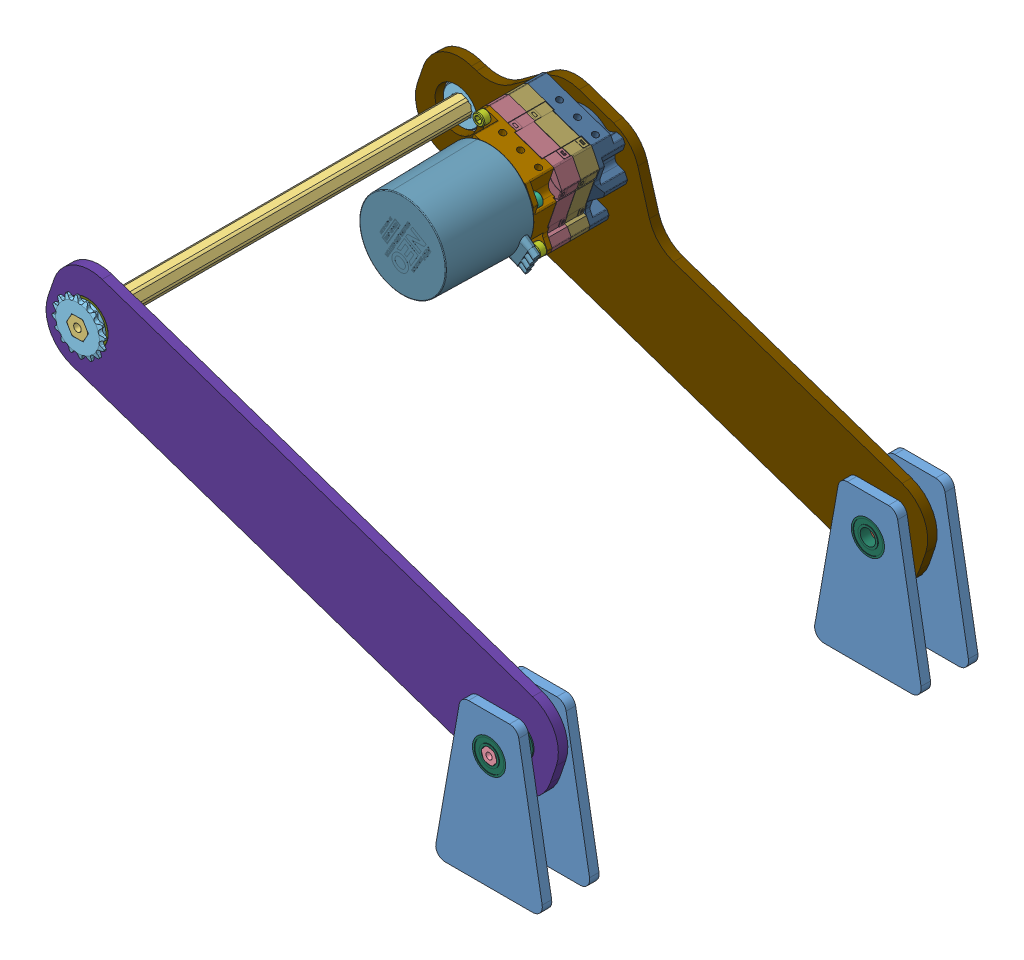
SolidWorks assembly intakeassembly, configuration Default. Lengths in mm.
Overall size (371.43 254.48 292.1).
35 component instances, 18 part files, 50 mates.
Components (placement in the parent):
- layout_sketch (2)-2: layout_sketch (2) [Default] at (16.0396 36.7133 123.2199) size (71.49 101.6 6.35)
- layout_sketch (2)-3: layout_sketch (2) [Default] at (16.0396 36.7133 -99.0301) size (71.49 101.6 6.35)
- 1_2thunderhex_1.5in-1: 1_2thunderhex_1.5in [Default] at (53.0044 112.9133 -556.2301) x (-0.618535 -0.785757 0) z (0 0 1) size (13.74 12.75 31.75)
- 1_2thunderhex_10.5in-1: 1_2thunderhex_10.5in [Default] at (-235.6241 210.8757 -308.5801) x (-0.456167 0.889894 0) z (0 0 1) size (13.74 12.75 266.7)
- 3_8thunderhex_1.5in-1: 3_8thunderhex_1.5in [Default] at (53.0044 112.9133 -295.8801) x (0.332678 -0.943041 0) z (0 0 1) size (10.24 9.53 38.1)
- 16T_#25_500_hex_hubbed_sprocket_217-2642-1: 16T_#25_500_hex_hubbed_sprocket_217-2642 [Default] at (-235.6241 210.8757 145.8259) x (-0.877701 0.479208 0) z (0 0 1) size (35.21 35.21 9.18)
- MAXPlanetary 2-Stage-1: MAXPlanetary 2-Stage [Default] at (-149.8677 235.4157 -51.4051) x (-0.946944 0.321399 0) z (0 0 -1) size (89.61 89.51 122.08)
  - MAXPlanetary 2-Stage.STEP-1: MAXPlanetary 2-Stage.STEP [Default] at origin size (89.61 89.51 122.08)
    - REV-25-2109_2-Stage (No Shaft, For NEO).STEP-1: REV-25-2109_2-Stage (No Shaft, For NEO).STEP [Default] at origin size (65.15 54.03 73.34)
      - REV-25-2107_2-Stage.STEP-1: REV-25-2107_2-Stage.STEP [Default] at (0 0 6.35) x (-1 0 0) z (0 0 -1) size (65.15 54.03 73.34)
        - #10 Socket Head Cap Screws_0.500in Long.STEP-1: #10 Socket Head Cap Screws_0.500in Long.STEP [Default] at (21.1355 14.0872 12.7) x (0.923728 0.383049 0) z (0.383049 -0.923728 0) size (7.94 17.53 7.94)
        - #10 Socket Head Cap Screws_0.500in Long.STEP-2: #10 Socket Head Cap Screws_0.500in Long.STEP [Default] at (-21.1355 -14.0872 12.7) x (0.923728 0.383049 0) z (0.383049 -0.923728 0) size (7.94 17.53 7.94)
        - #10 Socket Head Cap Screws_1.500in Long.STEP-1: #10 Socket Head Cap Screws_1.500in Long.STEP [Default] at (-26.9919 21.4312 0) x (0.777574 0.628792 0) z (-0.628792 0.777574 0) size (7.94 42.93 7.94)
        - #10 Socket Head Cap Screws_1.500in Long.STEP-2: #10 Socket Head Cap Screws_1.500in Long.STEP [Default] at (26.9919 -21.4312 0) x (0.777574 0.628792 0) z (-0.628792 0.777574 0) size (7.94 42.93 7.94)
        - #10-32 Button Head Cap Screws_0.500in Long.STEP-1: #10-32 Button Head Cap Screws_0.500in Long.STEP [Default] at (0 0 -35.2425) x (0.655967 -0.754789 0) z (-0.754789 -0.655967 0) size (9.17 15.27 9.17)
      - REV-21-2106.STEP-1: REV-21-2106.STEP [Default] at origin size (61.91 50.8 19.05)
      - REV-21-2104.STEP-1: REV-21-2104.STEP [Default] at (0 0 44.45) x (0 0 1) z (-1 0 0) size (23.2 50.8 61.92)
      - REV-21-2108.STEP-1: REV-21-2108.STEP [Default] at (0 0 7.0985) x (-0.554615 -0.832107 0) z (0 0 -1) size (25.4 25.4 14.94)
    - REV-21-2101.STEP-1: REV-21-2101.STEP [Default] at (0 0 28.575) size (61.91 50.8 16.85)
    - REV-21-2102.STEP-1: REV-21-2102.STEP [Default] at (0 0 15.875) size (61.91 50.8 16.85)
    - REV-21-1650.STEP-1: REV-21-1650.STEP [Default] at (0 0 -9.525) x (0.554615 0.832107 0) z (0 0 1) size (64.41 64.76 93.26)
- thunderhex_375_flanged_217-5829-1: thunderhex_375_flanged_217-5829 [Default] at (53.0044 112.9133 154.2079) x (0 0 1) z (-0.756545 -0.653942 0) size (7.11 24.61 24.61)
- thunderhex_375_flanged_217-5829-2: thunderhex_375_flanged_217-5829 [Default] at (53.0044 112.9133 -123.6681) x (0 0 -1) z (-0.718679 0.695342 0) size (7.11 24.61 24.61)
- thunderhex_flanged_217-4006-2: thunderhex_flanged_217-4006 [Default] at (-235.6241 210.8757 138.3012) x (-1 0 0) z (0 0 -1) size (31.12 31.12 7.94)
- layout_sketch (2)-4: layout_sketch (2) [Default] at (16.0396 36.7133 154.9699) size (71.49 101.6 6.35)
- layout_sketch (2)-5: layout_sketch (2) [Default] at (16.0396 36.7133 -130.7801) size (71.49 101.6 6.35)
- thunderhex_375_flanged_217-5829-3: thunderhex_375_flanged_217-5829 [Default] at (53.0044 112.9133 130.3319) x (0 0 -1) z (-0.959715 -0.280976 0) size (7.11 24.61 24.61)
- thunderhex_375_flanged_217-5829-5: thunderhex_375_flanged_217-5829 [Default] at (53.0044 112.9133 -99.7921) x (0 0 1) z (-0.999866 -0.016349 0) size (7.11 24.61 24.61)
- thunderhex_375_flanged_217-5829-6: thunderhex_375_flanged_217-5829 [Default] at (53.0044 112.9133 135.9199) x (0 0 1) z (-0.999379 0.03525 0) size (7.11 24.61 24.61)
- thunderhex_375_flanged_217-5829-7: thunderhex_375_flanged_217-5829 [Default] at (53.0044 112.9133 -105.3801) x (0 0 -1) z (-0.879404 0.476076 0) size (7.11 24.61 24.61)
- layout_sketch (1)-1: layout_sketch (1) [Default] at (63.5174 28.8757 142.2699) x (-0.946944 0.321399 0) z (0 0 -1) size (355.6 63.5 6.35)
- layout_sketch-1: layout_sketch [Default] at (63.5174 28.8757 -105.3801) x (-0.946944 0.321399 0) z (0 0 -1) size (355.6 107.95 6.35)
- 16T_#25_500_hex_hubbed_sprocket_217-2642-2: 16T_#25_500_hex_hubbed_sprocket_217-2642 [Default] at (-235.6241 210.8757 -115.2861) x (-1 0 0) z (0 0 -1) size (35.21 35.21 9.18)
- 16T_#25_500_hex_hubbed_sprocket_217-2642-3: 16T_#25_500_hex_hubbed_sprocket_217-2642 [Default] at (-149.8677 235.4157 -115.2861) x (-0.723016 -0.690831 0) z (0 0 -1) size (35.21 35.21 9.18)
- 1_2thunderhex_1.5in-2: 1_2thunderhex_1.5in [Default] at (-149.8677 235.4157 -543.5301) x (0.99729 -0.073573 0) z (0 0 1) size (13.74 12.75 31.75)
Mates (geometry in assembly coordinates):
- Parallel1: parallel aligned: line of layout_sketch (2)-2 through (23.6073 36.7133 129.5699) axis (1 0 0); line of layout_sketch (2)-3 through (23.6073 36.7133 -92.6801) axis (1 0 0)
- Parallel3: parallel aligned: plane of layout_sketch (2)-2 through (39.2827 138.3133 129.5699) normal (0 1 0); plane of layout_sketch (2)-3 through (39.2827 138.3133 -92.6801) normal (0 1 0)
- Distance1: distance = 222.25 mm aligned: plane of layout_sketch (2)-3 through (82.4016 43.0633 -92.6801) normal (0 0 1); plane of layout_sketch (2)-2 through (82.4016 43.0633 129.5699) normal (0 0 1)
- Coincident3: coincident aligned: plane of layout_sketch (2)-2 through (39.2827 138.3133 129.5699) normal (0 1 0); plane of layout_sketch (2)-3 through (39.2827 138.3133 -92.6801) normal (0 1 0)
- Coincident4: coincident aligned: plane of layout_sketch (2)-2 through (72.9797 133.0659 129.5699) normal (0.984808 0.173648 0); plane of layout_sketch (2)-3 through (72.9797 133.0659 -92.6801) normal (0.984808 0.173648 0)
- Parallel6: parallel aligned: plane of layout_sketch (2)-2 through (39.2827 138.3133 129.5699) normal (0 1 0); plane of layout_sketch (2)-4 through (39.2827 138.3133 161.3199) normal (0 1 0)
- Parallel7: parallel aligned: plane of layout_sketch (2)-2 through (72.9797 133.0659 129.5699) normal (0.984808 0.173648 0); plane of layout_sketch (2)-4 through (72.9797 133.0659 161.3199) normal (0.984808 0.173648 0)
- Coincident14: coincident aligned: plane of layout_sketch (2)-2 through (72.9797 133.0659 129.5699) normal (0.984808 0.173648 0); plane of layout_sketch (2)-4 through (72.9797 133.0659 161.3199) normal (0.984808 0.173648 0)
- Coincident15: coincident aligned: plane of layout_sketch (2)-2 through (39.2827 138.3133 129.5699) normal (0 1 0); plane of layout_sketch (2)-4 through (39.2827 138.3133 161.3199) normal (0 1 0)
- Coincident16: coincident aligned: plane of layout_sketch (2)-3 through (39.2827 138.3133 -92.6801) normal (0 1 0); plane of layout_sketch (2)-5 through (39.2827 138.3133 -124.4301) normal (0 1 0)
- Coincident17: coincident aligned: plane of layout_sketch (2)-3 through (72.9797 133.0659 -92.6801) normal (0.984808 0.173648 0); plane of layout_sketch (2)-5 through (72.9797 133.0659 -124.4301) normal (0.984808 0.173648 0)
- Coincident20: coincident aligned: plane of layout_sketch (2)-3 through (82.4016 43.0633 -92.6801) normal (0 0 1); plane of thunderhex_375_flanged_217-5829-5 through (52.8425 122.8179 -92.6801) normal (0 0 1)
- Concentric9: concentric aligned: cylinder of layout_sketch (2)-3 through (53.0044 112.9133 -92.6801) axis (0 0 -1) radius 11.1125; cylinder of thunderhex_375_flanged_217-5829-5 through (53.0044 112.9133 -99.7921) axis (0 0 -1) radius 5.125
- Coincident23: coincident aligned: plane of thunderhex_375_flanged_217-5829-2 through (46.1164 105.794 -130.7801) normal (0 0 -1); plane of layout_sketch (2)-5 through (82.4016 43.0633 -130.7801) normal (0 0 -1)
- Concentric10: concentric anti-aligned: cylinder of thunderhex_375_flanged_217-5829-2 through (53.0044 112.9133 -123.6681) axis (0 0 1) radius 5.125; cylinder of layout_sketch (2)-5 through (53.0044 112.9133 -124.4301) axis (0 0 -1) radius 11.1125
- Coincident27: coincident aligned: plane of layout_sketch (2)-2 through (82.4016 43.0633 123.2199) normal (0 0 -1); plane of thunderhex_375_flanged_217-5829-3 through (55.7878 103.4063 123.2199) normal (0 0 -1)
- Concentric13: concentric anti-aligned: cylinder of layout_sketch (2)-2 through (53.0044 112.9133 129.5699) axis (0 0 -1) radius 11.1125; cylinder of thunderhex_375_flanged_217-5829-3 through (53.0044 112.9133 130.3319) axis (0 0 1) radius 5.125
- Coincident31: coincident aligned: plane of thunderhex_375_flanged_217-5829-1 through (46.5265 120.4076 161.3199) normal (0 0 1); plane of layout_sketch (2)-4 through (82.4016 43.0633 161.3199) normal (0 0 1)
- Concentric15: concentric anti-aligned: cylinder of thunderhex_375_flanged_217-5829-1 through (53.0044 112.9133 154.2079) axis (0 0 -1) radius 5.125; circle of layout_sketch (2)-4
- Distance2: distance = 31.75 mm aligned: plane of layout_sketch (2)-2 through (82.4016 43.0633 129.5699) normal (0 0 1); plane of layout_sketch (2)-4 through (82.4016 43.0633 161.3199) normal (0 0 1)
- Distance3: distance = 31.75 mm aligned: plane of layout_sketch (2)-5 through (82.4016 43.0633 -124.4301) normal (0 0 1); plane of layout_sketch (2)-3 through (82.4016 43.0633 -92.6801) normal (0 0 1)
- Coincident34: coincident aligned: plane of 3_8thunderhex_1.5in-1 through (53.0044 112.9133 161.3199) normal (0 0 1); plane of layout_sketch (2)-4 through (82.4016 43.0633 161.3199) normal (0 0 1)
- Concentric16: concentric anti-aligned: cylinder of 3_8thunderhex_1.5in-1 through (53.0044 112.9133 -753.0801) axis (0 0 1) radius 2.1; cylinder of thunderhex_375_flanged_217-5829-1 through (53.0044 112.9133 154.2079) axis (0 0 -1) radius 5.125
- Coincident36: coincident aligned: plane of 1_2thunderhex_1.5in-1 through (88.5441 168.3684 -130.7801) normal (0 0 -1); plane of layout_sketch (2)-5 through (82.4016 43.0633 -130.7801) normal (0 0 -1)
- Concentric17: concentric aligned: cylinder of 1_2thunderhex_1.5in-1 through (53.0044 112.9133 -1013.4301) axis (0 0 1) radius 2.55; cylinder of thunderhex_375_flanged_217-5829-2 through (53.0044 112.9133 -123.6681) axis (0 0 1) radius 5.125
- Concentric18: concentric aligned: cylinder of 1_2thunderhex_1.5in-1 through (53.0044 112.9133 -1013.4301) axis (0 0 1) radius 2.55; cylinder of thunderhex_375_flanged_217-5829-7 through (53.0044 112.9133 -105.3801) axis (0 0 1) radius 5.125
- Concentric19: concentric anti-aligned: cylinder of 3_8thunderhex_1.5in-1 through (53.0044 112.9133 -753.0801) axis (0 0 1) radius 2.1; cylinder of thunderhex_375_flanged_217-5829-6 through (53.0044 112.9133 135.9199) axis (0 0 -1) radius 5.125
- Distance6: distance = 12.7 mm aligned: plane of thunderhex_375_flanged_217-5829-7 through (47.1457 102.0911 -105.3801) normal (0 0 1); plane of layout_sketch (2)-3 through (82.4016 43.0633 -92.6801) normal (0 0 1)
- Distance7: distance = 12.7 mm aligned: plane of layout_sketch (2)-2 through (82.4016 43.0633 123.2199) normal (0 0 -1); plane of thunderhex_375_flanged_217-5829-6 through (53.4382 125.2119 135.9199) normal (0 0 -1)
- Concentric20: concentric aligned: cylinder of thunderhex_375_flanged_217-5829-7 through (53.0044 112.9133 -105.3801) axis (0 0 1) radius 11.1125; cylinder of layout_sketch-1 through (53.0044 112.9133 -111.7301) axis (0 0 1) radius 11.1125
- Concentric21: concentric aligned: cylinder of 3_8thunderhex_1.5in-1 through (53.0044 112.9133 -753.0801) axis (0 0 1) radius 2.1; cylinder of layout_sketch (1)-1 through (53.0044 112.9133 135.9199) axis (0 0 1) radius 11.1125
- Parallel9: parallel aligned: plane of layout_sketch (1)-1 through (63.2089 142.9787 135.9199) normal (0.321399 0.946944 0); plane of layout_sketch-1 through (63.2089 142.9787 -111.7301) normal (0.321399 0.946944 0)
- Coincident47: coincident aligned: plane of thunderhex_375_flanged_217-5829-6 through (53.4382 125.2119 135.9199) normal (0 0 -1); plane of layout_sketch (1)-1 through (-237.6649 204.8626 135.9199) normal (0 0 -1)
- Coincident48: coincident aligned: plane of thunderhex_375_flanged_217-5829-7 through (47.1457 102.0911 -105.3801) normal (0 0 1); plane of layout_sketch-1 through (-237.6649 204.8626 -105.3801) normal (0 0 1)
- Concentric23: concentric aligned: cylinder of 1_2thunderhex_10.5in-1 through (-235.6241 210.8757 -765.7801) axis (0 0 1) radius 2.55; cylinder of layout_sketch (1)-1 through (-235.6241 210.8757 135.9199) axis (0 0 1) radius 14.2875
- Distance8: distance = 6.35 mm aligned: plane of 1_2thunderhex_10.5in-1 through (-235.6241 210.8757 148.6199) normal (0 0 1); plane of layout_sketch (1)-1 through (-237.6649 204.8626 142.2699) normal (0 0 1)
- Coincident51: coincident aligned: plane of thunderhex_flanged_217-4006-2 through (-235.6241 223.1632 142.2699) normal (0 0 1); plane of layout_sketch (1)-1 through (-237.6649 204.8626 142.2699) normal (0 0 1)
- Concentric24: concentric anti-aligned: cylinder of thunderhex_flanged_217-4006-2 through (-235.6241 210.8757 85.0522) axis (0 0 -1) radius 6.875; cylinder of layout_sketch (1)-1 through (-235.6241 210.8757 135.9199) axis (0 0 1) radius 14.2875
- Concentric26: concentric anti-aligned: cylinder of 16T_#25_500_hex_hubbed_sprocket_217-2642-1 through (-235.6241 210.8757 139.4442) axis (0 0 1) radius 12.7; cylinder of thunderhex_flanged_217-4006-2 through (-235.6241 210.8757 85.0522) axis (0 0 -1) radius 14.2875
- Concentric27: concentric aligned: circle of 16T_#25_500_hex_hubbed_sprocket_217-2642-1; circle of thunderhex_flanged_217-4006-2
- Coincident53: coincident aligned: plane of 1_2thunderhex_10.5in-1 through (-235.6241 210.8757 148.6199) normal (0 0 1); plane of 16T_#25_500_hex_hubbed_sprocket_217-2642-1 through (-235.6241 210.8757 148.6199) normal (0 0 1)
- Concentric28: concentric anti-aligned: cylinder of 1_2thunderhex_10.5in-1 through (-235.6241 210.8757 -765.7801) axis (0 0 1) radius 2.55; cylinder of 16T_#25_500_hex_hubbed_sprocket_217-2642-2 through (-235.6241 210.8757 -108.9043) axis (0 0 -1) radius 12.7
- Coincident55: coincident aligned: plane of 1_2thunderhex_10.5in-1 through (-200.0458 155.4454 -118.0801) normal (0 0 -1); plane of 16T_#25_500_hex_hubbed_sprocket_217-2642-2 through (-235.6241 210.8757 -118.0801) normal (0 0 -1)
- Coincident56: coincident anti-aligned: plane of MAXPlanetary 2-Stage-1/MAXPlanetary 2-Stage.STEP-1/REV-25-2109_2-Stage (No Shaft, For NEO).STEP-1/REV-21-2104.STEP-1 through (-149.8677 235.4157 -105.3801) normal (0 0 -1); plane of layout_sketch-1 through (-237.6649 204.8626 -105.3801) normal (0 0 1)
- Parallel10: parallel aligned: plane of MAXPlanetary 2-Stage-1/MAXPlanetary 2-Stage.STEP-1/REV-25-2109_2-Stage (No Shaft, For NEO).STEP-1/REV-21-2104.STEP-1 through (-165.7565 267.6316 -86.3301) normal (0.321399 0.946944 0); plane of layout_sketch-1 through (63.2089 142.9787 -111.7301) normal (0.321399 0.946944 0)
- Concentric29: concentric aligned: cylinder of MAXPlanetary 2-Stage-1/MAXPlanetary 2-Stage.STEP-1/REV-25-2109_2-Stage (No Shaft, For NEO).STEP-1/REV-25-2107_2-Stage.STEP-1/#10-32 Button Head Cap Screws_0.500in Long.STEP-1 through (-149.8677 235.4157 -92.3753) axis (0 0 1) radius 2.413; cylinder of layout_sketch-1 through (-149.8677 235.4157 -111.7301) axis (0 0 1) radius 12.7
- Coincident58: coincident aligned: plane of 1_2thunderhex_10.5in-1 through (-200.0458 155.4454 -118.0801) normal (0 0 -1); plane of 1_2thunderhex_1.5in-2 through (-215.7158 233.8807 -118.0801) normal (0 0 -1)
- Concentric30: concentric aligned: cylinder of MAXPlanetary 2-Stage-1/MAXPlanetary 2-Stage.STEP-1/REV-25-2109_2-Stage (No Shaft, For NEO).STEP-1/REV-25-2107_2-Stage.STEP-1/#10-32 Button Head Cap Screws_0.500in Long.STEP-1 through (-149.8677 235.4157 -92.3753) axis (0 0 1) radius 2.413; cylinder of 1_2thunderhex_1.5in-2 through (-149.8677 235.4157 -1000.7301) axis (0 0 1) radius 2.55
- Coincident59: coincident aligned: plane of 16T_#25_500_hex_hubbed_sprocket_217-2642-2 through (-235.6241 210.8757 -118.0801) normal (0 0 -1); plane of 16T_#25_500_hex_hubbed_sprocket_217-2642-3 through (-149.8677 235.4157 -118.0801) normal (0 0 -1)
- Concentric31: concentric anti-aligned: cylinder of 16T_#25_500_hex_hubbed_sprocket_217-2642-3 through (-149.8677 235.4157 -108.9043) axis (0 0 -1) radius 12.7; cylinder of 1_2thunderhex_1.5in-2 through (-149.8677 235.4157 -1000.7301) axis (0 0 1) radius 2.55
